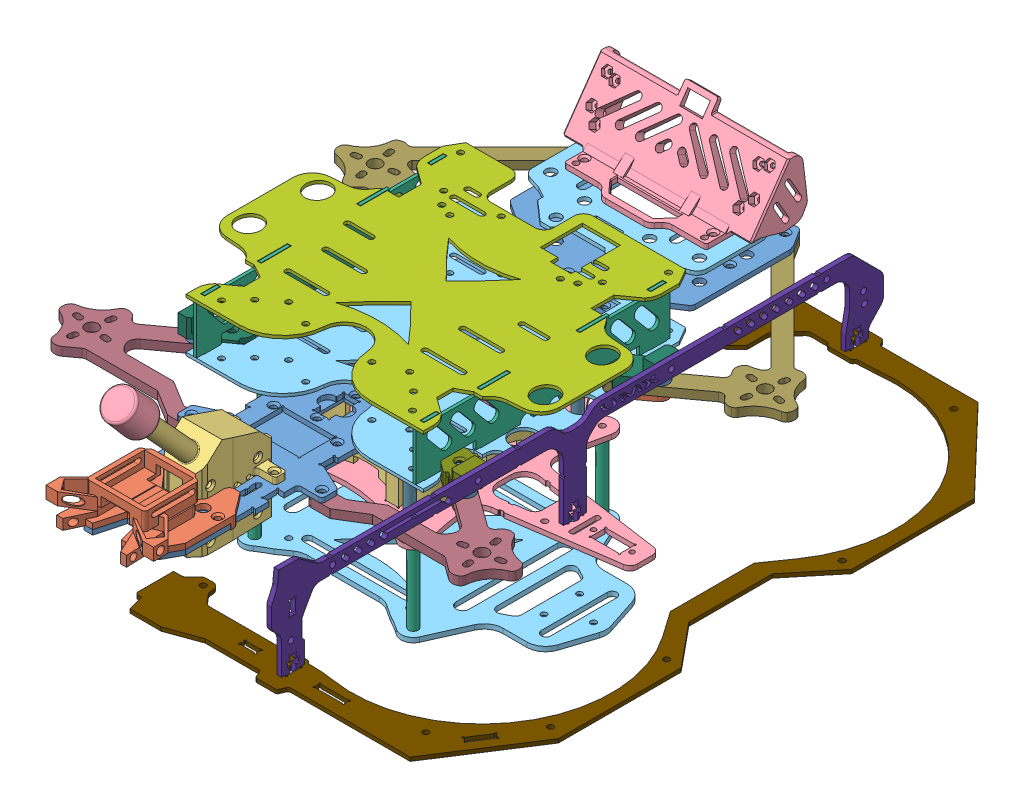
SolidWorks assembly 【Router】Chimera_5_XMU, configuration 默认. Lengths in mm.
Overall size (348.29 148.9 341.57).
197 component instances, 51 part files, 104 mates.
Components (placement in the parent):
- 主结构1-1: 主结构1 [默认] at (1.5044 -10.0257 329.067) size (150.98 2.73 325.31)
- 主结构2-1: 主结构2 [默认] at (1.5044 -14.5257 329.067) x (1 0 0) z (0 -1 0) size (150.98 112.29 2.5)
- [打印]飞塔保护壳-1: [打印]飞塔保护壳 [默认] at (1.5044 -17.0257 329.067) size (76.01 41.7 83)
- 底板_1-1: 底板_1 [默认] at (1.5044 -47.5257 329.067) size (209.17 2.5 135.35)
- 电池板SLDPRT-1: 电池板SLDPRT [默认] at (1.5044 -90.0257 329.067) size (187.98 2.5 112.92)
- 铝柱_40mm-5: 铝柱_40mm [默认] at (43.5044 -87.5257 279.067) x (0.657496 0 -0.753458) z (0 1 0) size (5 5 40)
- 铝柱_40mm-8: 铝柱_40mm [默认] at (-40.4956 -87.5257 279.067) x (-0.934177 0 -0.35681) z (0 1 0) size (5 5 40)
- 铝柱_40mm-9: 铝柱_40mm [默认] at (-40.4956 -87.5257 379.067) x (-0.934177 0 -0.35681) z (0 1 0) size (5 5 40)
- 铝柱_40mm-10: 铝柱_40mm [默认] at (43.5044 -87.5257 379.067) x (-0.903539 0 -0.428507) z (0 1 0) size (5 5 40)
- Air Unit.step-1: Air Unit.step [默认] at (8.357 -13.0257 442.2598) x (0 -1 0) z (0 0 -1) size (30.99 15 32.5) (hidden)
  - Bottom Case.step-1: Bottom Case.step [默认] at origin size (30.5 3.8 32.5)
  - Mid Case.step-1: Mid Case.step [默认] at origin size (30.5 12 32.5)
  - Top Case.step-1: Top Case.step [默认] at origin size (30.99 7.25 32.5)
  - Internal.step-1: Internal.step [默认] at origin size (29.25 12.4 30.75)
  - Screws.step-1: Screws.step [默认] at origin size (28.5 14.75 28.5)
- F45A.STEP-1: F45A.STEP [默认] at (2.5197 -30.0482 327.7528) size (44 7.18 42)
  - F45A PCB.STEP-1: F45A PCB.STEP [默认] at origin size (44 3.01 42)
  - DF13-10P.STEP-1: DF13-10P.STEP [默认] at (3.125 2.88 -16.6) x (-1 0 0) z (0 0 -1) size (14.25 3.58 5.1)
  - Heat Sink.STEP-1: Heat Sink.STEP [默认] at (0 2.5 0) size (37 3 37)
  - TPH1R403NL.STEP-1: TPH1R403NL.STEP [默认] at (8.2237 -1 16.1) x (0 0 -1) z (-1 0 0) size (5.3 1 6)
  - TPH1R403NL.STEP-2: TPH1R403NL.STEP [默认] at (8.5237 -1 9.95) x (-1 0 0) z (0 0 1) size (5.3 1 6)
  - TPH1R403NL.STEP-3: TPH1R403NL.STEP [默认] at (14.6737 -1 9.0737) x (0 0 1) z (1 0 0) size (5.3 1 6)
  - TPH1R403NL.STEP-4: TPH1R403NL.STEP [默认] at (14.6737 -1 2.8237) x (0 0 1) z (1 0 0) size (5.3 1 6)
  - TPH1R403NL.STEP-5: TPH1R403NL.STEP [默认] at (-8.2237 -1 16.1) x (0 0 1) z (1 0 0) size (5.3 1 6)
  - TPH1R403NL.STEP-6: TPH1R403NL.STEP [默认] at (-14.6737 -1 2.8237) x (0 0 -1) z (-1 0 0) size (5.3 1 6)
  - TPH1R403NL.STEP-7: TPH1R403NL.STEP [默认] at (-14.6737 -1 9.0737) x (0 0 -1) z (-1 0 0) size (5.3 1 6)
  - TPH1R403NL.STEP-8: TPH1R403NL.STEP [默认] at (8.2237 -1 -16.1) x (0 0 -1) z (-1 0 0) size (5.3 1 6)
  - TPH1R403NL.STEP-9: TPH1R403NL.STEP [默认] at (14.6737 -1 -2.8237) x (0 0 1) z (1 0 0) size (5.3 1 6)
  - TPH1R403NL.STEP-10: TPH1R403NL.STEP [默认] at (14.6737 -1 -9.0737) x (0 0 1) z (1 0 0) size (5.3 1 6)
  - TPH1R403NL.STEP-11: TPH1R403NL.STEP [默认] at (-8.2237 -1 -16.1) x (0 0 1) z (1 0 0) size (5.3 1 6)
  - TPH1R403NL.STEP-12: TPH1R403NL.STEP [默认] at (-14.6737 -1 -2.8237) x (0 0 -1) z (-1 0 0) size (5.3 1 6)
  - TPH1R403NL.STEP-13: TPH1R403NL.STEP [默认] at (-14.6737 -1 -9.0737) x (0 0 -1) z (-1 0 0) size (5.3 1 6)
  - TPH1R403NL.STEP-14: TPH1R403NL.STEP [默认] at (-8.5237 -1 9.95) x (-1 0 0) z (0 0 1) size (5.3 1 6)
  - TPH1R403NL.STEP-15: TPH1R403NL.STEP [默认] at (-8.5237 -1 -9.95) x (1 0 0) z (0 0 -1) size (5.3 1 6)
  - TPH1R403NL.STEP-16: TPH1R403NL.STEP [默认] at (8.5237 -1 -9.95) x (1 0 0) z (0 0 -1) size (5.3 1 6)
  - Capacitor.STEP-1: Capacitor.STEP [默认] at (9.5737 -1 -1.95) x (-1 0 0) z (0 0 1) size (3.2 1.5 1.6)
  - Capacitor.STEP-2: Capacitor.STEP [默认] at (9.5737 -1 -0.15) x (-1 0 0) z (0 0 1) size (3.2 1.5 1.6)
  - Capacitor.STEP-3: Capacitor.STEP [默认] at (9.5737 -1 1.65) x (-1 0 0) z (0 0 1) size (3.2 1.5 1.6)
  - Capacitor.STEP-4: Capacitor.STEP [默认] at (9.5737 -1 3.45) x (-1 0 0) z (0 0 1) size (3.2 1.5 1.6)
  - Capacitor.STEP-5: Capacitor.STEP [默认] at (-9.5737 -1 -1.95) x (-1 0 0) z (0 0 1) size (3.2 1.5 1.6)
  - Capacitor.STEP-6: Capacitor.STEP [默认] at (-9.5737 -1 -0.15) x (-1 0 0) z (0 0 1) size (3.2 1.5 1.6)
  - Capacitor.STEP-7: Capacitor.STEP [默认] at (-9.5737 -1 1.65) x (-1 0 0) z (0 0 1) size (3.2 1.5 1.6)
  - Capacitor.STEP-8: Capacitor.STEP [默认] at (-9.5737 -1 3.45) x (-1 0 0) z (0 0 1) size (3.2 1.5 1.6)
  - Capacitor.STEP-9: Capacitor.STEP [默认] at (5.3737 -1.8 -8.35) x (0 0 1) z (0 -1 0) size (3.2 1.5 1.6)
  - Capacitor.STEP-10: Capacitor.STEP [默认] at (3.5737 -1.8 -8.35) x (0 0 1) z (0 -1 0) size (3.2 1.5 1.6)
  - Capacitor.STEP-11: Capacitor.STEP [默认] at (1.7737 -1.8 -8.35) x (0 0 1) z (0 -1 0) size (3.2 1.5 1.6)
  - Capacitor.STEP-12: Capacitor.STEP [默认] at (-0.0263 -1.8 -8.35) x (0 0 1) z (0 -1 0) size (3.2 1.5 1.6)
  - Capacitor.STEP-13: Capacitor.STEP [默认] at (-1.8263 -1.8 -8.35) x (0 0 1) z (0 -1 0) size (3.2 1.5 1.6)
  - Capacitor.STEP-14: Capacitor.STEP [默认] at (5.3737 -1.8 10.75) x (0 0 1) z (0 -1 0) size (3.2 1.5 1.6)
  - Capacitor.STEP-15: Capacitor.STEP [默认] at (3.5737 -1.8 10.75) x (0 0 1) z (0 -1 0) size (3.2 1.5 1.6)
  - Capacitor.STEP-16: Capacitor.STEP [默认] at (1.7737 -1.8 10.75) x (0 0 1) z (0 -1 0) size (3.2 1.5 1.6)
  - Capacitor.STEP-17: Capacitor.STEP [默认] at (-0.0263 -1.8 10.75) x (0 0 1) z (0 -1 0) size (3.2 1.5 1.6)
  - Capacitor.STEP-18: Capacitor.STEP [默认] at (-1.8263 -1.8 10.75) x (0 0 1) z (0 -1 0) size (3.2 1.5 1.6)
  - Capacitor.STEP-19: Capacitor.STEP [默认] at (-4.4263 -2.5 10.75) x (0 0 1) z (-1 0 0) size (3.2 1.5 1.6)
- [云台板]思翼A8Mini-1: [云台板]思翼A8Mini [默认] at (1.5044 54.4743 329.0671) x (-1 0 -0.000003) z (0 -1 0) size (92.34 65.32 2) (hidden)
- 机臂2-1: 机臂2 [默认] at (1.5044 -10.0257 329.067) x (1 0 0) z (0 0 -1) size (93.94 4.5 157.55)
- 机臂2-3: 机臂2 [默认] at (1.5044 -14.5257 329.067) x (-1 0 0) z (0 0 -1) size (93.94 4.5 157.55)
- 机臂3-1: 机臂3 [默认] at (1.5044 -14.5257 329.067) size (93.8 4.5 97.35)
- 机臂3-2: 机臂3 [默认] at (1.5044 -10.0257 329.067) x (-1 0 0) z (0 0 1) size (93.8 4.5 97.35)
- 铝柱_35mm-1: 铝柱_35mm [默认] at (-30.4956 -10.0257 371.067) x (1 0 0) z (0 -1 0) size (5 5 35)
- 铝柱_35mm-2: 铝柱_35mm [默认] at (33.5044 -10.0257 371.067) x (1 0 0) z (0 -1 0) size (5 5 35)
- 铝柱_35mm-3: 铝柱_35mm [默认] at (-34.4956 -10.0257 286.067) x (1 0 0) z (0 -1 0) size (5 5 35)
- 铝柱_35mm-4: 铝柱_35mm [默认] at (37.5044 -10.0257 286.067) x (1 0 0) z (0 -1 0) size (5 5 35)
- [打印]防撞圈安装件-右前左后_安装调整-1: [打印]防撞圈安装件-右前左后_安装调整 [默认] at (61.729 -7.5257 285.3113) size (22.94 14.75 21.64) (hidden)
- [打印]防撞圈安装件-右前左后_安装调整-2: [打印]防撞圈安装件-右前左后_安装调整 [默认] at (-58.7202 -7.5257 372.8227) x (-1 0 0) z (0 0 -1) size (22.94 14.75 21.64)
- [打印]防撞圈安装件-左前右后_安装调整-1: [打印]防撞圈安装件-左前右后_安装调整 [默认] at (-58.7202 -7.5257 285.3113) size (22.94 14.75 21.64)
- [打印]防撞圈安装件-左前右后_安装调整-2: [打印]防撞圈安装件-左前右后_安装调整 [默认] at (61.729 -7.5257 372.8227) x (-1 0 0) z (0 0 -1) size (22.94 14.75 21.64) (hidden)
- 防撞圈固定板-1: 防撞圈固定板 [默认] at (76.5044 3.7243 329.067) x (0 0 -1) z (1 0 0) size (323.84 57.5 2.5)
- 防撞圈-2片式-1: 防撞圈-2片式 [默认] at (1.5044 -42.0257 329.067) x (0 0 -1) z (0 1 0) size (322.86 178.56 2)
- [pcb]分电PCB轮廓-1: [pcb]分电PCB轮廓 [默认] at (1.5044 -11.6257 337.2797) size (53.58 3 152.15)
- [打印]综合天线接口-5寸机_修改-1: [打印]综合天线接口-5寸机_修改 [默认] at (1.5044 -7.5257 329.067) size (57 20.5 61.52)
- [打印]o3支架-1: [打印]o3支架 [默认] at (1.5044 -13.0257 329.067) size (40.8 71.3 61.95)
- Antenna.step-1: Antenna.step [默认] at (1.5044 5.6745 451.7025) x (-0.985663 0.113991 -0.124399) z (0 -0.737277 -0.67559) size (17.31 17.31 63)
- 铝柱_30mm-1: 铝柱_30mm [默认] at (40.8394 -10.0257 208.8847) x (1 0 0) z (0 -1 0) size (5 5 30) (hidden)
- 铝柱_30mm-2: 铝柱_30mm [默认] at (16.1053 -10.0257 462.8732) x (-0.837169 0 -0.546944) z (0 -1 0) size (5 5 30) (hidden)
- [云台板]G-port云台结构-1: [云台板]G-port云台结构 [默认] at (1.5041 3.4743 329.0669) x (-1 0 -0.000003) z (0 -1 0) size (92.34 65.32 2)
- [打印]飞控转接板-1: [打印]飞控转接板 [默认] at (1.5044 -36.7457 329.067) x (1 0 0) z (0 -1 0) size (36.5 36.5 2)
- [云台板]astrorc单轴云台-2: [云台板]astrorc单轴云台 [默认] at (1.5044 0.9743 329.067) x (-1 0 0) z (0 -1 0) size (92.34 58.82 29.5) (hidden)
- MTF-01 Optical Flow &Lidar Sensor.step-1: MTF-01 Optical Flow &Lidar Sensor.step [默认] at (-13.1758 -52.2597 251.4922) x (0.999998 0 -0.002058) z (0 -1 0) size (29.45 17.1 14.23)
  - Board.step-1: Board.step [默认] at origin size (29.45 17.1 1.28)
    - Open CASCADE STEP translator 6.8 1.1.1.step-1: Open CASCADE STEP translator 6.8 1.1.1.step [默认] at (0 0 -1.279) size (29.45 17.1 1.28)
  - Open CASCADE STEP translator 6.8 1.2.step-1: Open CASCADE STEP translator 6.8 1.2.step [默认] at origin size (6 4.95 2.96)
    - SM04B-SRSS-TB.step-1: SM04B-SRSS-TB.step [默认] at (11.4779 13.1201 -0.979) x (1 0 0) z (0 1 0) size (6 2.96 4.95)
  - U5.step-1: U5.step [默认] at origin size (4.09 4.09 0.8)
    - QFN50P400X400X80-25N.step-1: QFN50P400X400X80-25N.step [默认] at (14.3501 5.7301 -1.279) x (0 -1 0) z (0 0 -1) size (4.09 4.09 0.8)
  - R17.step-1: R17.step [默认] at origin size (0.55 1.05 0.4)
    - RES_0402_(1005_metric).step-1: RES_0402_(1005_metric).step [默认] at (16.5751 15.6 -1.279) x (0 1 0) z (0 0 -1) size (1.05 0.55 0.4)
  - R16.step-1: R16.step [默认] at origin size (0.55 1.05 0.4)
    - RES_0402_(1005_metric).step-1: RES_0402_(1005_metric).step [默认] at (15.6251 15.6 -1.279) x (0 1 0) z (0 0 -1) size (1.05 0.55 0.4)
  - R15.step-1: R15.step [默认] at origin size (1.05 0.55 0.4)
    - RES_0402_(1005_metric).step-1: RES_0402_(1005_metric).step [默认] at (23.05 13.1499 0) x (-1 0 0) z (0 0 1) size (1.05 0.55 0.4)
  - R14.step-1: R14.step [默认] at origin size (1.05 0.55 0.4)
    - RES_0402_(1005_metric).step-1: RES_0402_(1005_metric).step [默认] at (14.45 11.0499 -1.279) x (1 0 0) z (0 0 -1) size (1.05 0.55 0.4)
  - R13.step-1: R13.step [默认] at origin size (1.05 0.55 0.4)
    - RES_0402_(1005_metric).step-1: RES_0402_(1005_metric).step [默认] at (21.75 6.7499 -1.279) x (1 0 0) z (0 0 -1) size (1.05 0.55 0.4)
  - R12.step-1: R12.step [默认] at origin size (1.05 0.55 0.4)
    - RES_0402_(1005_metric).step-1: RES_0402_(1005_metric).step [默认] at (12.75 0.8501 0) x (1 0 0) z (0 0 1) size (1.05 0.55 0.4)
  - R11.step-1: R11.step [默认] at origin size (1.05 0.55 0.4)
    - RES_0402_(1005_metric).step-1: RES_0402_(1005_metric).step [默认] at (11.95 0.9499 -1.279) x (1 0 0) z (0 0 -1) size (1.05 0.55 0.4)
  - R10.step-1: R10.step [默认] at origin size (0.55 1.05 0.4)
    - RES_0402_(1005_metric).step-1: RES_0402_(1005_metric).step [默认] at (18.1001 4.675 -1.279) x (0 1 0) z (0 0 -1) size (1.05 0.55 0.4)
  - R9.step-1: R9.step [默认] at origin size (0.55 1.05 0.4)
    - RES_0402_(1005_metric).step-1: RES_0402_(1005_metric).step [默认] at (11.3001 8.6 -1.279) x (0 1 0) z (0 0 -1) size (1.05 0.55 0.4)
  - R8.step-1: R8.step [默认] at origin size (0.55 1.05 0.4)
    - RES_0402_(1005_metric).step-1: RES_0402_(1005_metric).step [默认] at (18.4501 9.65 -1.279) x (0 1 0) z (0 0 -1) size (1.05 0.55 0.4)
  - R7.step-1: R7.step [默认] at origin size (0.55 1.05 0.4)
    - RES_0402_(1005_metric).step-1: RES_0402_(1005_metric).step [默认] at (17.3501 9.65 -1.279) x (0 1 0) z (0 0 -1) size (1.05 0.55 0.4)
  - R6.step-1: R6.step [默认] at origin size (0.55 1.05 0.4)
    - RES_0402_(1005_metric).step-1: RES_0402_(1005_metric).step [默认] at (16.3501 9.65 -1.279) x (0 1 0) z (0 0 -1) size (1.05 0.55 0.4)
  - R5.step-1: R5.step [默认] at origin size (0.55 1.05 0.4)
    - RES_0402_(1005_metric).step-1: RES_0402_(1005_metric).step [默认] at (15.3501 9.65 -1.279) x (0 1 0) z (0 0 -1) size (1.05 0.55 0.4)
  - R4.step-1: R4.step [默认] at origin size (0.55 1.05 0.4)
    - RES_0402_(1005_metric).step-1: RES_0402_(1005_metric).step [默认] at (14.3501 9.65 -1.279) x (0 1 0) z (0 0 -1) size (1.05 0.55 0.4)
  - R3.step-1: R3.step [默认] at origin size (0.55 1.05 0.4)
    - RES_0402_(1005_metric).step-1: RES_0402_(1005_metric).step [默认] at (13.3501 9.65 -1.279) x (0 1 0) z (0 0 -1) size (1.05 0.55 0.4)
  - R2.step-1: R2.step [默认] at origin size (0.55 1.05 0.4)
    - RES_0402_(1005_metric).step-1: RES_0402_(1005_metric).step [默认] at (12.3501 9.65 -1.279) x (0 1 0) z (0 0 -1) size (1.05 0.55 0.4)
  - R1.step-1: R1.step [默认] at origin size (1.05 0.55 0.4)
    - RES_0402_(1005_metric).step-1: RES_0402_(1005_metric).step [默认] at (21.75 15.0501 0) x (1 0 0) z (0 0 1) size (1.05 0.55 0.4)
  - D3.step-1: D3.step [默认] at origin size (5.7 5.3 12.2)
    - LED_5mm______.step-1: LED_5mm______.step [默认] at (19.65 5.55 0) x (0 1 0) z (0 0 1) size (5.3 5.7 8.7)
    - LED_5MM-W.step-1: LED_5MM-W.step [默认] at (19.65 5.55 0) x (0 1 0) z (0 0 1) size (4.06 1.6 7.95)
  - D2.step-1: D2.step [默认] at origin size (5.7 5.3 12.2)
    - LED_5MM-R.step-1: LED_5MM-R.step [默认] at (9.65 5.55 0) x (0 -1 0) z (0 0 1) size (4.06 1.6 7.95)
      - LED_5MM-R-5814_AF0_ASM.step-1: LED_5MM-R-5814_AF0_ASM.step [默认] at origin size (4.06 1.6 7.95)
        - LED_5MM-R-936_AF0.step-1: LED_5MM-R-936_AF0.step [默认] at origin size (4.06 1.6 7.95)
    - LED_5mm______.step-1: LED_5mm______.step [默认] at (9.65 5.55 0) x (0 -1 0) z (0 0 1) size (5.3 5.7 8.7)
  - D1.step-1: D1.step [默认] at origin size (1.6 0.8 0.75)
    - LED_0603_APT1608_BLUE.step-1: LED_0603_APT1608_BLUE.step [默认] at (21.7501 16.1501 0) x (1 0 0) z (0 0 1) size (1.6 0.8 0.75)
  - C28.step-1: C28.step [默认] at origin size (0.55 1.05 0.55)
    - CAP_0402_(1005_metric).step-1: CAP_0402_(1005_metric).step [默认] at (8.3501 11.65 0) x (0 -1 0) z (0 0 1) size (1.05 0.55 0.55)
  - C27.step-1: C27.step [默认] at origin size (1.05 0.55 0.55)
    - CAP_0402_(1005_metric).step-1: CAP_0402_(1005_metric).step [默认] at (15.45 12.0499 -1.279) x (1 0 0) z (0 0 -1) size (1.05 0.55 0.55)
  - C26.step-1: C26.step [默认] at origin size (1.05 0.55 0.55)
    - CAP_0402_(1005_metric).step-1: CAP_0402_(1005_metric).step [默认] at (15.45 12.9501 -1.279) x (-1 0 0) z (0 0 -1) size (1.05 0.55 0.55)
  - C25.step-1: C25.step [默认] at origin size (1.05 0.55 0.55)
    - CAP_0402_(1005_metric).step-1: CAP_0402_(1005_metric).step [默认] at (9.85 13.5501 0) x (1 0 0) z (0 0 1) size (1.05 0.55 0.55)
  - C24.step-1: C24.step [默认] at origin size (0.9 1.7 0.9)
    - CAP_0603.step-1: CAP_0603.step [默认] at (9.8499 11.55 -0.013) x (0 1 0) z (0 0 1) size (1.7 0.9 0.9)
  - C23.step-1: C23.step [默认] at origin size (0.55 1.05 0.55)
    - CAP_0402_(1005_metric).step-1: CAP_0402_(1005_metric).step [默认] at (10.4499 15.35 0) x (0 1 0) z (0 0 1) size (1.05 0.55 0.55)
  - C21.step-1: C21.step [默认] at origin size (0.9 1.7 0.9)
    - CAP_0603.step-1: CAP_0603.step [默认] at (9.2499 15.55 -0.013) x (0 1 0) z (0 0 1) size (1.7 0.9 0.9)
  - C20.step-1: C20.step [默认] at origin size (0.55 1.05 0.55)
    - CAP_0402_(1005_metric).step-1: CAP_0402_(1005_metric).step [默认] at (15.5501 1.75 0) x (0 -1 0) z (0 0 1) size (1.05 0.55 0.55)
  - C19.step-1: C19.step [默认] at origin size (1.05 0.55 0.55)
    - CAP_0402_(1005_metric).step-1: CAP_0402_(1005_metric).step [默认] at (14.35 2.3501 -1.279) x (-1 0 0) z (0 0 -1) size (1.05 0.55 0.55)
  - C18.step-1: C18.step [默认] at origin size (0.9 1.7 0.9)
    - CAP_0603.step-1: CAP_0603.step [默认] at (14.4501 1.55 -0.013) x (0 -1 0) z (0 0 1) size (1.7 0.9 0.9)
  - C17.step-1: C17.step [默认] at origin size (1.7 0.9 0.9)
    - CAP_0603.step-1: CAP_0603.step [默认] at (14.5 1.0501 -1.266) x (-1 0 0) z (0 0 -1) size (1.7 0.9 0.9)
  - C16.step-1: C16.step [默认] at origin size (0.55 1.05 0.55)
    - CAP_0402_(1005_metric).step-1: CAP_0402_(1005_metric).step [默认] at (19.7501 1.95 -1.279) x (0 1 0) z (0 0 -1) size (1.05 0.55 0.55)
  - C15.step-1: C15.step [默认] at origin size (1.45 2.2 1.35)
    - CAP_0805.step-1: CAP_0805.step [默认] at (16.9501 1.8501 -1.266) x (0 1 0) z (0 0 -1) size (2.2 1.45 1.35)
  - C14.step-1: C14.step [默认] at origin size (0.9 1.7 0.9)
    - CAP_0603.step-1: CAP_0603.step [默认] at (18.5501 1.75 -1.266) x (0 1 0) z (0 0 -1) size (1.7 0.9 0.9)
  - C13.step-1: C13.step [默认] at origin size (1.7 0.9 0.9)
    - CAP_0603.step-1: CAP_0603.step [默认] at (11.65 2.4499 -1.266) x (1 0 0) z (0 0 -1) size (1.7 0.9 0.9)
  - C12.step-1: C12.step [默认] at origin size (1.05 0.55 0.55)
    - CAP_0402_(1005_metric).step-1: CAP_0402_(1005_metric).step [默认] at (23.05 12.0501 0) x (1 0 0) z (0 0 1) size (1.05 0.55 0.55)
  - C11.step-1: C11.step [默认] at origin size (1.05 0.55 0.55)
    - CAP_0402_(1005_metric).step-1: CAP_0402_(1005_metric).step [默认] at (19.25 16.3499 0) x (-1 0 0) z (0 0 1) size (1.05 0.55 0.55)
  - C10.step-1: C10.step [默认] at origin size (1.05 0.55 0.55)
    - CAP_0402_(1005_metric).step-1: CAP_0402_(1005_metric).step [默认] at (20.75 10.5499 0) x (-1 0 0) z (0 0 1) size (1.05 0.55 0.55)
  - C8.step-1: C8.step [默认] at origin size (1.7 0.9 0.9)
    - CAP_0603.step-1: CAP_0603.step [默认] at (7.15 15.6501 -0.013) x (1 0 0) z (0 0 1) size (1.7 0.9 0.9)
  - C7.step-1: C7.step [默认] at origin size (1.7 0.9 0.9)
    - CAP_0603.step-1: CAP_0603.step [默认] at (23.15 5.2501 -1.266) x (-1 0 0) z (0 0 -1) size (1.7 0.9 0.9)
  - C6.step-1: C6.step [默认] at origin size (1.05 0.55 0.55)
    - CAP_0402_(1005_metric).step-1: CAP_0402_(1005_metric).step [默认] at (23.25 10.8501 -1.279) x (-1 0 0) z (0 0 -1) size (1.05 0.55 0.55)
  - C5.step-1: C5.step [默认] at origin size (0.9 1.7 0.9)
    - CAP_0603.step-1: CAP_0603.step [默认] at (20.1499 9.5 -1.266) x (0 -1 0) z (0 0 -1) size (1.7 0.9 0.9)
  - C4.step-1: C4.step [默认] at origin size (0.9 1.7 0.9)
    - CAP_0603.step-1: CAP_0603.step [默认] at (10.0501 10.35 -1.266) x (0 1 0) z (0 0 -1) size (1.7 0.9 0.9)
  - C3.step-1: C3.step [默认] at origin size (0.55 1.05 0.55)
    - CAP_0402_(1005_metric).step-1: CAP_0402_(1005_metric).step [默认] at (8.6501 11.85 -1.279) x (0 1 0) z (0 0 -1) size (1.05 0.55 0.55)
  - C2.step-1: C2.step [默认] at origin size (0.55 1.05 0.55)
    - CAP_0402_(1005_metric).step-1: CAP_0402_(1005_metric).step [默认] at (7.1501 13.15 -1.279) x (0 1 0) z (0 0 -1) size (1.05 0.55 0.55)
  - C1.step-1: C1.step [默认] at origin size (0.9 1.7 0.9)
    - CAP_0603.step-1: CAP_0603.step [默认] at (5.9501 13.5 -1.266) x (0 1 0) z (0 0 -1) size (1.7 0.9 0.9)
  - Free-Models.step-1: Free-Models.step [默认] at origin size (18.05 14.8 10)
    - lens_chip_package.step-1: lens_chip_package.step [默认] at (14.7574 16.3068 -0.127) x (0 -1 0) z (-1 0 0) size (6 5.08 6)
      - LENS.step-1: LENS.step [默认] at origin size (3.8 3.95 3.8)
        - Open CASCADE STEP translator 6.8 1.50.3.1.1.step-1: Open CASCADE STEP translator 6.8 1.50.3.1.1.step [默认] at origin size (3.8 1.95 3.8)
        - Open CASCADE STEP translator 6.8 1.50.3.1.2.step-1: Open CASCADE STEP translator 6.8 1.50.3.1.2.step [默认] at origin size (2.37 3.08 2.37)
      - NONE.step-1: NONE.step [默认] at origin size (6 2.28 6)
    - ____&______.step-1: ____&______.step [默认] at (19.6718 5.5748 0) x (-1 0 0) z (0 0 -1) size (8 8 10)
    - ____&______.step-2: ____&______.step [默认] at (9.6266 5.524 0) x (-1 0 0) z (0 0 -1) size (8 8 10)
- 铝柱_40mm-11: 铝柱_40mm [默认] at (-85.7956 -47.5257 329.067) x (1 0 0) z (0 -1 0) size (5 5 40)
- [打印]G-port云台板双目接驳件-1: [打印]G-port云台板双目接驳件 [默认] at (1.5041 3.4743 329.0669) x (1 0 0.000003) z (0 1 0) size (100 46.6 38.07)
- [打印]防撞圈安装件-右前左后_安装调整-3: [打印]防撞圈安装件-右前左后_安装调整 [默认] at (61.729 -7.5307 285.3113) size (22.94 14.75 21.64)
- [打印]防撞圈安装件-左前右后_安装调整-3: [打印]防撞圈安装件-左前右后_安装调整 [默认] at (61.88 -7.5257 372.8227) x (-1 0 0) z (0 0 -1) size (22.94 14.75 21.64)
- Shell_Bottom_Router-1: Shell_Bottom_Router [Default] at (1.5044 -7.5257 339.5893) x (1 0 0) z (0 0 1) size (206.99 1.6 205.54)
- Shell_Side_X2_Router-1: Shell_Side_X2_Router [默认] at (58.7544 -5.9257 262.3393) x (1 0 0) z (0 0 1) size (1.6 28.2 134.5)
- Shell_Side_X2_Router-2: Shell_Side_X2_Router [默认] at (-57.3456 -5.9257 262.3393) x (1 0 0) z (0 0 1) size (1.6 28.2 134.5)
- Shell_Top_Router-1: Shell_Top_Router [Default] at (1.5044 19.0743 339.5893) x (1 0 0) z (0 0 1) size (194.24 1.6 181.57)
Mates (geometry in assembly coordinates):
- 同心75: concentric anti-aligned: cylinder of 主结构1-1 through (16.7544 -7.5257 313.817) axis (0 -1 0) radius 1.55; cylinder of 主结构2-1 through (16.7544 -17.0257 313.817) axis (0 1 0) radius 1.55
- 同心76: concentric anti-aligned: cylinder of 主结构1-1 through (-58.7202 -7.5257 372.8227) axis (0 -1 0) radius 1.55; cylinder of 机臂3-2 through (-58.7202 -14.5257 372.8227) axis (0 1 0) radius 1.55
- 重合80: coincident anti-aligned: plane of 主结构1-1 through (1.5044 -10.0257 113.8082) normal (0 -1 0); plane of 机臂3-2 through (-36.8355 -10.0257 356.9226) normal (0 1 0)
- 同心77: concentric anti-aligned: cylinder of 主结构1-1 through (61.729 -7.5257 285.3113) axis (0 -1 0) radius 1.55; cylinder of 机臂2-1 through (61.729 -14.5257 285.3113) axis (0 1 0) radius 1.55
- 同心78: concentric aligned: cylinder of 主结构1-1 through (45.5486 -7.5257 361.067) axis (0 -1 0) radius 1.55; cylinder of 机臂3-1 through (45.5486 -10.0257 361.067) axis (0 -1 0) radius 1.55
- 重合81: coincident anti-aligned: plane of 主结构2-1 through (1.5044 -14.5257 177.7429) normal (0 1 0); plane of 机臂3-1 through (39.8443 -14.5257 356.9226) normal (0 -1 0)
- 同心79: concentric anti-aligned: cylinder of 主结构2-1 through (-58.7202 -17.0257 372.8227) axis (0 1 0) radius 1.55; circle of 机臂3-2
- 重合83: coincident anti-aligned: plane of 主结构2-1 through (1.5044 -14.5257 177.7429) normal (0 1 0); plane of 机臂3-2 through (-36.8355 -14.5257 356.9226) normal (0 -1 0)
- 重合84: coincident anti-aligned: plane of 主结构2-1 through (1.5044 -14.5257 177.7429) normal (0 1 0); plane of 机臂2-3 through (1.5044 -14.5257 329.067) normal (0 -1 0)
- 同心80: concentric anti-aligned: cylinder of 主结构2-1 through (-58.7202 -17.0257 285.3113) axis (0 1 0) radius 1.55; cylinder of 机臂2-3 through (-58.7202 -10.0257 285.3113) axis (0 -1 0) radius 1.55
- 同心81: concentric anti-aligned: cylinder of 主结构2-1 through (-42.5398 -17.0257 297.067) axis (0 1 0) radius 1.55; cylinder of 机臂2-3 through (-42.5398 -10.0257 297.067) axis (0 -1 0) radius 1.55
- 同心82: concentric anti-aligned: cylinder of 主结构2-1 through (45.5486 -17.0257 361.067) axis (0 1 0) radius 1.55; cylinder of 机臂3-1 through (45.5486 -10.0257 361.067) axis (0 -1 0) radius 1.55
- 同心83: concentric anti-aligned: cylinder of 主结构2-1 through (61.729 -17.0257 372.8227) axis (0 1 0) radius 1.55; cylinder of 机臂3-1 through (61.729 -10.0257 372.8227) axis (0 -1 0) radius 1.55
- 重合85: coincident anti-aligned: plane of 主结构2-1 through (1.5044 -14.5257 177.7429) normal (0 1 0); plane of 机臂3-1 through (39.8443 -14.5257 356.9226) normal (0 -1 0)
- 同心84: concentric aligned: cylinder of 主结构1-1 through (45.5486 -7.5257 361.067) axis (0 -1 0) radius 1.55; cylinder of 机臂3-1 through (45.5486 -10.0257 361.067) axis (0 -1 0) radius 1.55
- 同心85: concentric aligned: cylinder of 主结构1-1 through (61.729 -7.5257 372.8227) axis (0 -1 0) radius 1.55; cylinder of 机臂3-1 through (61.729 -10.0257 372.8227) axis (0 -1 0) radius 1.55
- 重合86: coincident anti-aligned: plane of 主结构1-1 through (1.5044 -10.0257 113.8082) normal (0 -1 0); plane of 机臂3-1 through (39.8443 -10.0257 356.9226) normal (0 1 0)
- 同心86: concentric anti-aligned: cylinder of 主结构1-1 through (37.5044 -7.5257 286.067) axis (0 -1 0) radius 1.55; cylinder of 铝柱_35mm-4 through (37.5044 -45.0257 286.067) axis (0 1 0) radius 1.55
- 重合87: coincident anti-aligned: plane of 主结构1-1 through (1.5044 -10.0257 113.8082) normal (0 -1 0); plane of 铝柱_35mm-4 through (37.5044 -10.0257 286.067) normal (0 1 0)
- 同心87: concentric anti-aligned: cylinder of 主结构1-1 through (-34.4956 -7.5257 286.067) axis (0 -1 0) radius 1.55; cylinder of 铝柱_35mm-3 through (-34.4956 -45.0257 286.067) axis (0 1 0) radius 1.55
- 重合88: coincident anti-aligned: plane of 主结构1-1 through (1.5044 -10.0257 113.8082) normal (0 -1 0); plane of 铝柱_35mm-3 through (-34.4956 -10.0257 286.067) normal (0 1 0)
- 同心88: concentric anti-aligned: cylinder of 主结构1-1 through (-30.4956 -7.5257 371.067) axis (0 -1 0) radius 1.55; cylinder of 铝柱_35mm-1 through (-30.4956 -45.0257 371.067) axis (0 1 0) radius 1.55
- 重合89: coincident anti-aligned: plane of 主结构1-1 through (1.5044 -10.0257 113.8082) normal (0 -1 0); plane of 铝柱_35mm-1 through (-30.4956 -10.0257 371.067) normal (0 1 0)
- 同心89: concentric anti-aligned: cylinder of 主结构1-1 through (33.5044 -7.5257 371.067) axis (0 -1 0) radius 1.55; cylinder of 铝柱_35mm-2 through (33.5044 -45.0257 371.067) axis (0 1 0) radius 1.55
- 重合90: coincident anti-aligned: plane of 主结构1-1 through (1.5044 -10.0257 113.8082) normal (0 -1 0); plane of 铝柱_35mm-2 through (33.5044 -10.0257 371.067) normal (0 1 0)
- 同心90: concentric anti-aligned: cylinder of 底板_1-1 through (33.5044 -45.0257 371.067) axis (0 -1 0) radius 1.55; cylinder of 铝柱_35mm-2 through (33.5044 -45.0257 371.067) axis (0 1 0) radius 1.55
- 同心91: concentric anti-aligned: cylinder of 底板_1-1 through (-30.4956 -45.0257 371.067) axis (0 -1 0) radius 1.55; cylinder of 铝柱_35mm-1 through (-30.4956 -45.0257 371.067) axis (0 1 0) radius 1.55
- 重合91: coincident anti-aligned: plane of 底板_1-1 through (-244.6747 -45.0257 329.067) normal (0 1 0); plane of 铝柱_35mm-1 through (-30.4956 -45.0257 371.067) normal (0 -1 0)
- 距离1: distance = 3.75 mm anti-aligned: plane of Air Unit.step-1/Top Case.step-1 through (-6.143 -13.0257 442.2598) normal (-1 0 0); plane of 主结构1-1 through (-9.893 -7.5257 456.5808) normal (1 0 0)
- 重合95: coincident anti-aligned: plane of 底板_1-1 through (-244.6747 -47.5257 329.067) normal (0 -1 0); plane of 铝柱_40mm-9 through (-40.4956 -47.5257 379.067) normal (0 1 0)
- 重合96: coincident anti-aligned: plane of 底板_1-1 through (-244.6747 -47.5257 329.067) normal (0 -1 0); plane of 铝柱_40mm-10 through (43.5044 -47.5257 379.067) normal (0 1 0)
- 重合97: coincident anti-aligned: plane of 底板_1-1 through (-244.6747 -47.5257 329.067) normal (0 -1 0); plane of 铝柱_40mm-5 through (43.5044 -47.5257 279.067) normal (0 1 0)
- 重合99: coincident anti-aligned: plane of 底板_1-1 through (-244.6747 -47.5257 329.067) normal (0 -1 0); plane of 铝柱_40mm-8 through (-40.4956 -47.5257 279.067) normal (0 1 0)
- 重合100: coincident anti-aligned: plane of 电池板SLDPRT-1 through (1.5044 -87.5257 217.5353) normal (0 1 0); plane of 铝柱_40mm-8 through (-40.4956 -87.5257 279.067) normal (0 -1 0)
- 重合101: coincident anti-aligned: plane of 主结构1-1 through (1.5044 -7.5257 113.8082) normal (0 1 0); plane of [打印]防撞圈安装件-1 through (58.6606 -7.5257 287.5406) normal (0 -1 0)
- 同心93: concentric aligned: cylinder of 主结构1-1 through (61.729 -7.5257 285.3113) axis (0 -1 0) radius 1.55; cylinder of [打印]防撞圈安装件-1 through (61.729 -5.0257 285.3113) axis (0 -1 0) radius 1.55
- 同心96: concentric aligned: cylinder of 主结构1-1 through (-58.7202 -7.5257 372.8227) axis (0 -1 0) radius 1.55; cylinder of [打印]防撞圈安装件-右前左后-2 through (-58.7202 -5.0257 372.8227) axis (0 -1 0) radius 1.55
- 平行6: parallel aligned: plane of 主结构1-1 through (-56.2656 -7.5257 376.9106) normal (0.587785 0 0.809017); plane of [打印]防撞圈安装件-右前左后-2 through (-51.3904 -12.5257 376.4588) normal (0.587785 0 0.809017)
- 同心97: concentric aligned: cylinder of 主结构1-1 through (-58.7202 -7.5257 285.3113) axis (0 -1 0) radius 1.55; cylinder of [打印]防撞圈安装件-左前右后-1 through (-58.7202 -5.0257 285.3113) axis (0 -1 0) radius 1.55
- 平行7: parallel aligned: plane of 主结构1-1 through (-72.0294 -7.5257 281.5129) normal (-0.587785 0 0.809017); plane of [打印]防撞圈安装件-左前右后-1 through (-59.9132 -12.5257 293.4059) normal (-0.587785 0 0.809017)
- 重合103: coincident anti-aligned: plane of 主结构1-1 through (1.5044 -7.5257 113.8082) normal (0 1 0); plane of [打印]防撞圈安装件-左前右后-1 through (-55.6518 -7.5257 287.5406) normal (0 -1 0)
- 同心98: concentric aligned: cylinder of 主结构1-1 through (61.729 -7.5257 372.8227) axis (0 -1 0) radius 1.55; cylinder of [打印]防撞圈安装件-左前右后-2 through (61.729 -5.0257 372.8227) axis (0 -1 0) radius 1.55
- 平行8: parallel aligned: plane of 主结构1-1 through (59.2744 -7.5257 376.9106) normal (-0.587785 0 0.809017); plane of [打印]防撞圈安装件-左前右后-2 through (54.3992 -12.5257 376.4588) normal (-0.587785 0 0.809017)
- 重合105: coincident anti-aligned: plane of [打印]防撞圈安装件-左前右后-2 through (58.6606 -7.5257 370.5934) normal (0 -1 0); plane of 主结构1-1 through (1.5044 -7.5257 113.8082) normal (0 1 0)
- 距离2: distance = 0.15 mm anti-aligned: plane of 防撞圈固定板-1 through (79.0044 3.7243 329.067) normal (1 0 0); plane of 底板_1-1 through (79.1544 -45.0257 331.2188) normal (-1 0 0)
- 距离3: distance = 0.5 mm anti-aligned: plane of 防撞圈固定板-1 through (79.0044 -45.0257 325.567) normal (0 0 -1); plane of 底板_1-1 through (76.3544 -45.0257 325.067) normal (0 0 1)
- 重合108: coincident aligned: plane of 底板_1-1 through (-244.6747 -47.5257 329.067) normal (0 -1 0); plane of 防撞圈固定板-1 through (79.0044 -47.5257 327.517) normal (0 -1 0)
- 重合115: coincident anti-aligned: plane of 防撞圈固定板-1 through (79.0044 -40.0257 474.817) normal (0 -1 0); plane of 防撞圈-2片式-1 through (104.733 -40.0257 404.067) normal (0 1 0)
- 距离6: distance = 0.5 mm anti-aligned: plane of 防撞圈固定板-1 through (76.5044 3.7243 329.067) normal (-1 0 0); plane of 防撞圈-2片式-1 through (76.0044 -40.0257 183.817) normal (1 0 0)
- 距离5: distance = 0.5 mm anti-aligned: plane of 防撞圈固定板-1 through (79.0044 -40.0257 176.317) normal (0 0 -1); plane of 防撞圈-2片式-1 through (76.0044 -40.0257 175.817) normal (0 0 1)
- 同心99: concentric aligned: cylinder of 主结构1-1 through (1.5044 -7.5257 388.067) axis (0 -1 0) radius 1.55; cylinder of [pcb]分电PCB轮廓-1 through (1.5044 -10.0257 388.067) axis (0 -1 0) radius 1.55
- 同心100: concentric aligned: cylinder of 主结构1-1 through (1.5044 -7.5257 367.567) axis (0 -1 0) radius 1.55; cylinder of [pcb]分电PCB轮廓-1 through (1.5044 -10.0257 367.567) axis (0 -1 0) radius 1.55
- 重合116: coincident anti-aligned: plane of 主结构1-1 through (1.5044 -7.5257 113.8082) normal (0 1 0); plane of [打印]综合天线接口-5寸机-1 through (-6.518 -7.5257 452.8141) normal (0 -1 0)
- 同心101: concentric aligned: cylinder of 主结构1-1 through (-20.8855 -7.5257 462.8732) axis (0 -1 0) radius 1.55; cylinder of [打印]综合天线接口-5寸机-1 through (-20.8855 -4.5257 462.8732) axis (0 -1 0) radius 1.55
- 距离7: distance = 1 mm anti-aligned: plane of [打印]o3支架-1 through (1.5044 -31.2757 421.7598) normal (0 0 -1); plane of 主结构1-1 through (-7.9956 -7.5257 420.7598) normal (0 0 1)
- 距离8: distance = 0.5 mm anti-aligned: plane of 主结构1-1 through (12.8999 -7.5257 452.7032) normal (-0.999459 0 0.032881); plane of [打印]o3支架-1 through (8.3248 -31.2757 328.8426) normal (0.999459 0 -0.032881)
- 平行10: parallel anti-aligned: plane of 主结构1-1 through (-9.8911 -7.5257 452.7032) normal (0.999459 0 0.032881); plane of [打印]o3支架-1 through (-5.3159 -31.2757 328.8426) normal (-0.999459 0 -0.032881)
- 平行11: parallel anti-aligned: plane of [打印]o3支架-1 through (1.5044 36.9862 480.3945) normal (0 0.737277 0.67559); plane of Antenna.step-1 through (0.223 5.8227 451.5408) normal (0 -0.737277 -0.67559)
- 同心104: concentric anti-aligned: circle of Antenna.step-1; circle of [打印]o3支架-1
- 同心106: concentric aligned: circle of Air Unit.step-1/Screws.step-1; circle of [打印]o3支架-1
- 同心107: concentric anti-aligned: circle of Air Unit.step-1/Screws.step-1; circle of [打印]o3支架-1
- 重合125: coincident anti-aligned: plane of [打印]o3支架-1 through (1.5044 36.9862 480.3945) normal (0 0.737277 0.67559); circle of Antenna.step-1
- 重合126: coincident anti-aligned: plane of 主结构1-1 through (1.5044 -7.5257 113.8082) normal (0 1 0); plane of [打印]o3支架-1 through (1.5044 -7.5257 329.067) normal (0 -1 0)
- 重合127: coincident anti-aligned: plane of 主结构1-1 through (1.5044 -10.0257 113.8082) normal (0 -1 0); plane of 铝柱_30mm-2 through (16.1053 -10.0257 462.8732) normal (0 1 0)
- 同心108: concentric anti-aligned: cylinder of 主结构1-1 through (16.1053 -7.5257 462.8732) axis (0 -1 0) radius 1.55; cylinder of 铝柱_30mm-2 through (16.1053 -40.0257 462.8732) axis (0 1 0) radius 1.55
- 同心109: concentric anti-aligned: cylinder of 主结构1-1 through (40.8394 -7.5257 208.8847) axis (0 -1 0) radius 1.55; cylinder of 铝柱_30mm-1 through (40.8394 -40.0257 208.8847) axis (0 1 0) radius 1.55
- 重合128: coincident anti-aligned: plane of 主结构1-1 through (1.5044 -10.0257 113.8082) normal (0 -1 0); plane of 铝柱_30mm-1 through (40.8394 -10.0257 208.8847) normal (0 1 0)
- 距离10: distance = 60 mm anti-aligned: plane of 主结构1-1 through (1.5044 -7.5257 113.8082) normal (0 1 0); plane of [云台板]思翼A8Mini-1 through (-43.145 52.4743 231.4462) normal (0 -1 0)
- 同心110: concentric anti-aligned: circle of 主结构1-1; circle of [云台板]思翼A8Mini-1
- 同心111: concentric anti-aligned: circle of 主结构1-1; circle of [云台板]思翼A8Mini-1
- 同心113: concentric aligned: circle of [云台板]思翼A8Mini-1; circle of [云台板]G-port云台结构-1
- 同心114: concentric aligned: circle of [云台板]思翼A8Mini-1; circle of [云台板]G-port云台结构-1
- 平行15: parallel anti-aligned: plane of 主结构2-1 through (1.5044 -17.0257 177.7429) normal (0 -1 0); plane of 飞控转接板-1 through (-13.7456 -36.7457 344.317) normal (0 1 0)
- 同心116: concentric aligned: circle of 主结构2-1; circle of 飞控转接板-1
- 同心117: concentric aligned: circle of 主结构2-1; circle of 飞控转接板-1
- 平行17: parallel aligned: plane of 主结构1-1 through (1.5044 -7.5257 113.8082) normal (0 1 0); plane of [云台板]astrorc单轴云台-2 through (-120.6097 0.9743 212.9405) normal (0 1 0)
- 同心120: concentric anti-aligned: circle of 主结构1-1; circle of [云台板]astrorc单轴云台-2
- 同心121: concentric anti-aligned: circle of 主结构1-1; circle of [云台板]astrorc单轴云台-2
- 同心122: concentric anti-aligned: circle of 底板_1-1; circle of 电池板SLDPRT-1
- 同心123: concentric aligned: circle of 底板_1-1; circle of 电池板SLDPRT-1
- 同心139: concentric anti-aligned: cylinder of 底板_1-1 through (-85.7956 -45.0257 329.067) axis (0 -1 0) radius 1.55; cylinder of 铝柱_40mm-11 through (-85.7956 -87.5257 329.067) axis (0 1 0) radius 1.55
- 重合133: coincident anti-aligned: plane of 电池板SLDPRT-1 through (1.5044 -87.5257 217.5353) normal (0 1 0); plane of 铝柱_40mm-11 through (-85.7956 -87.5257 329.067) normal (0 -1 0)
- 距离14: distance = 6.5 mm anti-aligned: plane of [云台板]astrorc单轴云台-2 through (-120.6097 -1.0257 212.9405) normal (0 -1 0); plane of 主结构1-1 through (1.5044 -7.5257 113.8082) normal (0 1 0)
- 距离17: distance = 9 mm anti-aligned: plane of 主结构1-1 through (1.5044 -7.5257 113.8082) normal (0 1 0); plane of [云台板]G-port云台结构-1 through (-39.3801 1.4743 227.9) normal (0 -1 0)
- 同心150: concentric anti-aligned: cylinder of [云台板]G-port云台结构-1 through (-32.5455 1.4743 212.4845) axis (0 1 0) radius 1.55; cylinder of [打印]G-port云台板双目接驳件-1 through (-32.5455 6.2243 212.4845) axis (0 -1 0) radius 1.55
- 重合140: coincident anti-aligned: plane of [云台板]G-port云台结构-1 through (-39.3801 3.4743 227.9) normal (0 1 0); plane of [打印]G-port云台板双目接驳件-1 through (1.5041 3.4743 329.0669) normal (0 -1 0)
- 同心151: concentric anti-aligned: cylinder of [云台板]G-port云台结构-1 through (35.5545 1.4743 212.4847) axis (0 1 0) radius 1.55; cylinder of [打印]G-port云台板双目接驳件-1 through (35.5545 6.2243 212.4847) axis (0 -1 0) radius 1.55
- 重合144: coincident anti-aligned: cylinder of 防撞圈固定板-1 through (79.0044 -1.7757 380.1785) axis (-1 0 0) radius 1.55; circle of [打印]防撞圈安装件-左前右后_安装调整-3
- 同心159: concentric anti-aligned: cylinder of 底板_1-1 through (13.6544 44.3658 253.987) axis (0 -1 0) radius 1.925; cylinder of MTF-01 Optical Flow &Lidar Sensor.step-1/Board.step-1/Open CASCADE STEP translator 6.8 1.1.1.step-1 through (13.6544 -50.9807 253.987) axis (0 1 0) radius 1.25
- 距离18: distance = 0.5 mm: line of MTF-01 Optical Flow &Lidar Sensor.step-1/Open CASCADE STEP translator 6.8 1.2.step-1/SM04B-SRSS-TB.step-1 through (0.8284 -48.0257 264.2284) axis (-0.999998 0 0.002058); plane of 底板_1-1 through (-244.6747 -47.5257 329.067) normal (0 -1 0)
- 重合145: coincident anti-aligned: plane of 主结构1-1 through (1.5044 -7.5257 113.8082) normal (0 1 0); plane of [打印]防撞圈安装件-右前左后_安装调整-2 through (-55.6518 -7.5257 370.5934) normal (0 -1 0)
- 同心160: concentric aligned: cylinder of 主结构1-1 through (61.729 -7.5257 285.3113) axis (0 -1 0) radius 1.55; cylinder of [打印]防撞圈安装件-右前左后_安装调整-3 through (61.729 -5.0307 285.3113) axis (0 -1 0) radius 1.55
- Concentric2: concentric aligned: circle of 主结构1-1; circle of Shell_Bottom_Router-1
- Concentric1: concentric aligned: cylinder of 主结构1-1 through (19.0044 -7.5257 376.567) axis (0 -1 0) radius 1.55; circle of Shell_Bottom_Router-1
- Coincident4: coincident anti-aligned: plane of 主结构1-1 through (1.5044 -7.5257 113.8082) normal (0 1 0); plane of Shell_Bottom_Router-1 through (1.5044 -7.5257 339.5893) normal (0 -1 0)
- Distance1: distance = 0.25 mm anti-aligned: plane of Shell_Side_X2_Router-1 through (60.3544 -5.9257 262.3393) normal (1 0 0); plane of Shell_Bottom_Router-1 through (60.6044 -5.9257 339.5893) normal (-1 0 0)
- Coincident6: coincident: plane of Shell_Bottom_Router-1 through (1.5044 -5.9257 339.5893) normal (0 1 0); line of Shell_Side_X2_Router-1 through (60.3544 -5.9257 276.2749) axis (0 0 -1)
- Distance3: distance = 0.25 mm anti-aligned: plane of Shell_Bottom_Router-1 through (1.5044 -5.9257 262.0893) normal (0 0 1); plane of Shell_Side_X2_Router-1 through (60.3544 -5.9257 262.3393) normal (0 0 -1)
- Distance4: distance = 0.25 mm anti-aligned: plane of Shell_Side_X2_Router-2 through (-55.7456 -5.9257 262.3393) normal (1 0 0); plane of Shell_Bottom_Router-1 through (-55.4956 -5.9257 339.5893) normal (-1 0 0)
- Coincident9: coincident anti-aligned: plane of Shell_Bottom_Router-1 through (1.5044 -5.9257 339.5893) normal (0 1 0); plane of Shell_Side_X2_Router-2 through (-55.7456 -5.9257 262.3393) normal (0 -1 0)
- Distance5: distance = 0.25 mm anti-aligned: plane of Shell_Side_X2_Router-2 through (-55.7456 -5.9257 270.3393) normal (0 0 1); plane of Shell_Bottom_Router-1 through (1.5044 -5.9257 270.5893) normal (0 0 -1)
- Coincident11: coincident: plane of Shell_Side_X2_Router-2 through (-55.7456 19.0743 262.3393) normal (0 1 0); plane of Shell_Top_Router-1 through (1.5044 19.0743 339.5893) normal (0 -1 0)
- Distance6: distance = 0.25 mm: plane of Shell_Top_Router-1 through (-55.4956 20.6743 339.5893) normal (-1 0 0); plane of Shell_Side_X2_Router-2 through (-55.7456 -5.9257 262.3393) normal (1 0 0)
- Distance7: distance = 0.25 mm anti-aligned: plane of Shell_Top_Router-1 through (1.5044 20.6743 270.5893) normal (0 0 -1); plane of Shell_Side_X2_Router-2 through (-55.7456 19.0743 270.3393) normal (0 0 1)
